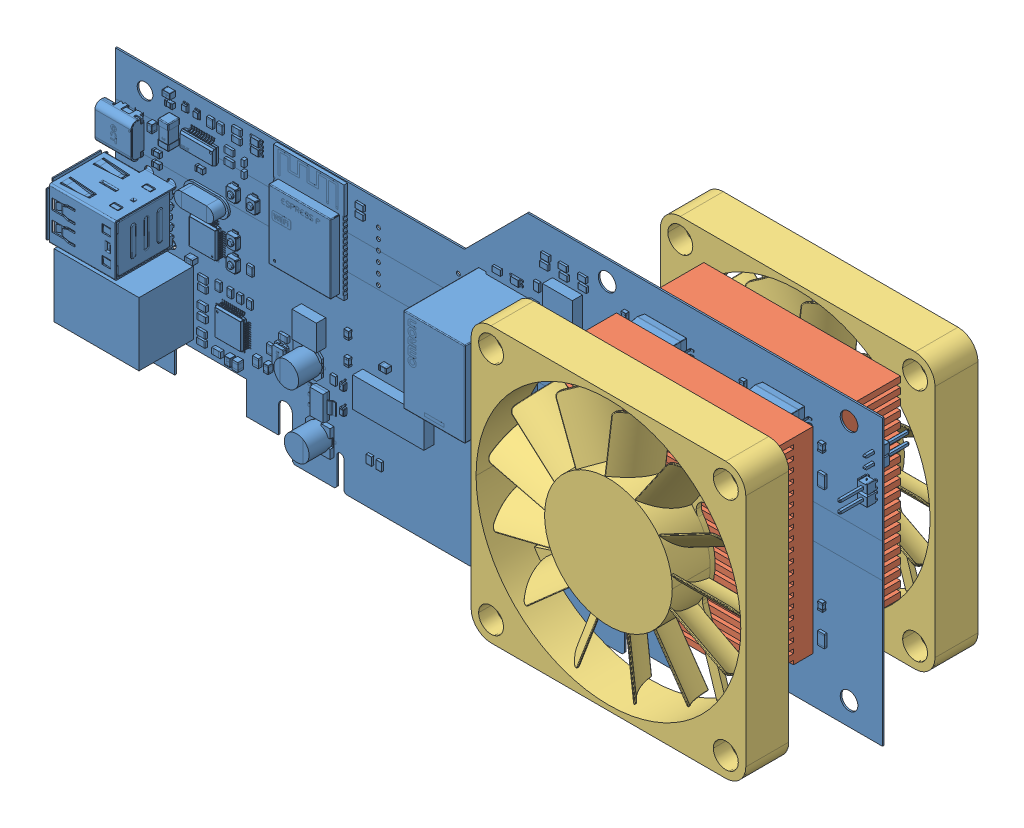
SolidWorks assembly ANTS_DCU_B1_Assembly, configuration Default. Lengths in mm.
Overall size (196.79 85.24 59.04).
5 component instances, 3 part files, 3 mates.
Components (placement in the parent):
- ANTS-DCU_RevB1-1: ANTS-DCU_RevB1 [Default] at origin size (196.79 85.17 38.29)
- DCU-heatsink-1: DCU-heatsink [Default] at (155.9769 52.9293 3.6) size (50 50 15)
- DCU-heatsink-2: DCU-heatsink [Default] at (155.9769 52.9293 -3.6) x (-1 0 0) z (0 0 -1) size (50 50 15)
- 70x15mm_fan-1: 70x15mm_fan [Default] at (119.92 15.23 29.522) size (69.85 69.85 10.92)
- 70x15mm_fan-4: 70x15mm_fan [Default] at (119.92 15.23 -18.6) size (69.85 69.85 10.92)
Mates (geometry in assembly coordinates):
- Coincident1: coincident anti-aligned: plane of ANTS-DCU_RevB1-1 through (145.55 43 3.6) normal (0 0 1); plane of DCU-heatsink-1 through (155.9769 52.9293 3.6) normal (0 0 -1)
- Coincident2: coincident anti-aligned: plane of DCU-heatsink-1 through (155.9769 52.9293 18.6) normal (0 0 1); plane of 70x15mm_fan-1 through (184.69 20.31 18.6) normal (0 0 -1)
- Concentric1: concentric aligned: cylinder of ANTS-DCU_RevB1-1 through (125 80 -0.4103) axis (0 0 -1) radius 2.25; circle of 70x15mm_fan-1
